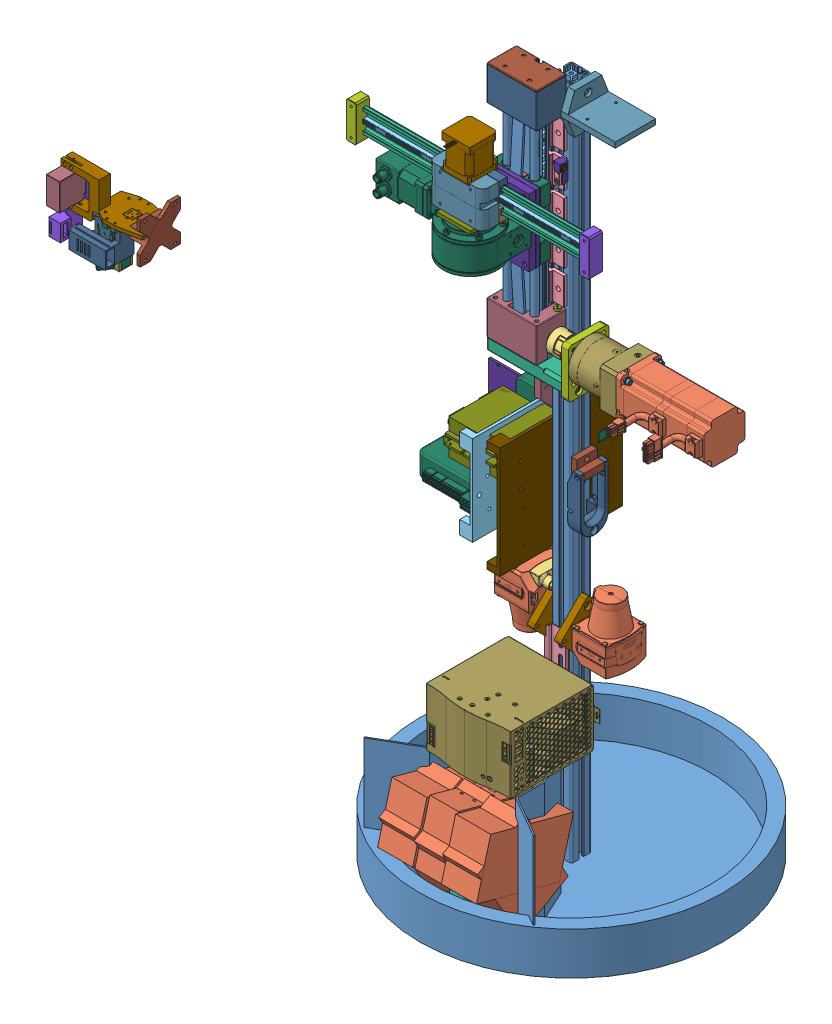
SolidWorks assembly Igus Axes Assembly, configuration Default. Lengths in mm.
Overall size (1488.85 1013 1350).
212 component instances, 89 part files, 64 mates.
Components (placement in the parent):
- Item Profile 6-1: Item Profile 6 [Default] at (483.1878 96.2857 998.7104) size (30 1000 30)
- TIM551 Lidar-1: TIM551 Lidar [Default] at (543.1878 396.2857 1000.2581) size (85.26 98.36 61.15)
  - TIM551 Lidar.igs-1: TIM551 Lidar.igs [Default] at origin size (85.26 98.36 61.15)
    - Assembly1.igs-1: Assembly1.igs [Default] at origin size (85.26 98.36 61.15)
      - 9194920_TiM55._56._35._36._Dummy.igs-1: 9194920_TiM55._56._35._36._Dummy.igs [Default] at origin size (85.26 98.36 61.15)
        - S105071_TiM55x_Mantelteile.igs-1: S105071_TiM55x_Mantelteile.igs [Default] at (11.3439 3.1936 0) x (0 1 0) z (0 0 -1) size (98.36 71.39 61.15)
        - S105072_TiM55x_Steckeranschluss_Dummy.igs-1: S105072_TiM55x_Steckeranschluss_Dummy.igs [Default] at (52.6134 34.7282 -20.9281) x (-1 0 0.000098) z (0.000098 -0.000098 1) size (37.21 29.83 42.7)
- Z Axis-1: Z Axis [Default] at (453.5786 1106.2857 1013.5104) x (1 0 0) z (0 -1 0) size (331.51 109.68 369.54)
  - D00684285.STEP-1: D00684285.STEP [Default] at origin size (331.51 109.68 369.54)
    - D00424608.iam.STEP-1: D00424608.iam.STEP [Default] at (0 0 52) x (-1 0 0) z (0 0 -1) size (74 44 56)
      - D00418189.iam.STEP-1: D00418189.iam.STEP [Default] at (0 22 30) x (-1 0 0) z (0 0 1) size (71 40 33.5)
        - D00160580.ipt.STEP-1: D00160580.ipt.STEP [Default] x (0 0 -1) z (-1 0 0) size (23 23 67.7)
        - D00129954.ipt.STEP-1: D00129954.ipt.STEP [Default] at (-25.5 0 0) x (0 1 0) z (-1 0 0) size (40 30 10)
        - D00129954.ipt.STEP-2: D00129954.ipt.STEP [Default] at (25.5 0 0) x (0 -1 0) z (1 0 0) size (40 30 10)
        - D00130409.ipt.STEP-1: D00130409.ipt.STEP [Default] at (-33.5 0 0) x (0 0 1) z (1 0 0) size (26 26 8)
        - D00130409.ipt.STEP-2: D00130409.ipt.STEP [Default] at (33.5 0 0) x (0 0 -1) z (-1 0 0) size (26 26 8)
        - D00130495.ipt.STEP-1: D00130495.ipt.STEP [Default] at (30.5 -15.5 -15) x (0 0 1) z (-1 0 0) size (23.5 8.5 8.5)
        - D00130495.ipt.STEP-2: D00130495.ipt.STEP [Default] at (-30.5 -15.5 -15) x (0 0 1) z (-1 0 0) size (23.5 8.5 8.5)
        - D00130495.ipt.STEP-3: D00130495.ipt.STEP [Default] at (-30.5 15.5 -15) x (0 0 1) z (-1 0 0) size (23.5 8.5 8.5)
        - D00130495.ipt.STEP-4: D00130495.ipt.STEP [Default] at (30.5 15.5 -15) x (0 0 1) z (1 0 0) size (23.5 8.5 8.5)
        - D00111820.ipt.STEP-1: D00111820.ipt.STEP [Default] at (-30.5 15.5 6.5896) x (0 0 1) z (1 0 0) size (5 5 5)
        - D00111820.ipt.STEP-2: D00111820.ipt.STEP [Default] at (-30.5 -15.5 6.5896) x (0 0 1) z (-1 0 0) size (5 5 5)
        - D00111820.ipt.STEP-3: D00111820.ipt.STEP [Default] at (30.5 -15.5 6.5896) x (0 0 1) z (-1 0 0) size (5 5 5)
        - D00111820.ipt.STEP-4: D00111820.ipt.STEP [Default] at (30.5 15.5 6.5896) x (0 0 1) z (-1 0 0) size (5 5 5)
      - D00129171.ipt.STEP-1: D00129171.ipt.STEP [Default] at (15 23.25 12) x (0 0 -1) z (1 0 0) size (18.8 7 7)
      - D00129171.ipt.STEP-2: D00129171.ipt.STEP [Default] at (-15 23.25 12) x (0 0 -1) z (1 0 0) size (18.8 7 7)
      - D00131296.ipt.STEP-1: D00131296.ipt.STEP [Default] x (-1 0 0) z (0 0 -1) size (74 44 50)
      - SAXT-104002.STEP-1: SAXT-104002.STEP [Default] at (0 22 52) x (-1 0 0) z (0 0 -1) size (74 44 7)
    - D00419202.iam.STEP-1: D00419202.iam.STEP [Default] at (0 0 302) size (94 44 56)
      - D00417520.iam.STEP-1: D00417520.iam.STEP [Default] at (0 22 25) x (-1 0 0) z (0 0 1) size (92.5 40 30)
        - D00130409.ipt.STEP-1: D00130409.ipt.STEP [Default] at (-25.5 0 0) x (0 -0.119291 0.992859) z (-1 0 0) size (26 26 8)
        - D00130409.ipt.STEP-2: D00130409.ipt.STEP [Default] at (33.5 0 0) x (0 0 -1) z (-1 0 0) size (26 26 8)
        - D00129954.ipt.STEP-1: D00129954.ipt.STEP [Default] at (-25.5 0 0) x (0 1 0) z (-1 0 0) size (40 30 10)
        - D00129954.ipt.STEP-2: D00129954.ipt.STEP [Default] at (25.5 0 0) x (0 -1 0) z (1 0 0) size (40 30 10)
        - D00160618.ipt.STEP-1: D00160618.ipt.STEP [Default] x (0 0 1) z (-1 0 0) size (23 23 90.85)
      - D00129171.ipt.STEP-1: D00129171.ipt.STEP [Default] at (15 23.25 12) x (0 0 -1) z (1 0 0) size (18.8 7 7)
      - D00129171.ipt.STEP-2: D00129171.ipt.STEP [Default] at (-15 23.25 12) x (0 0 -1) z (1 0 0) size (18.8 7 7)
      - D00130495.ipt.STEP-1: D00130495.ipt.STEP [Default] at (-30.5 6.5 0) x (0 0 1) z (-1 0 0) size (23.5 8.5 8.5)
      - D00130495.ipt.STEP-2: D00130495.ipt.STEP [Default] at (30.5 6.5 0) x (0 0 1) z (-1 0 0) size (23.5 8.5 8.5)
      - D00131302.ipt.STEP-1: D00131302.ipt.STEP [Default] x (-1 0 0) z (0 0 -1) size (74 44 50)
      - SAXT-104002_1.STEP-1: SAXT-104002_1.STEP [Default] at (0 22 52) x (-1 0 0) z (0 0 -1) size (74 44 24.04)
    - D00132325.iam.STEP-1: D00132325.iam.STEP [Default] at (0 30 177) size (73 22.56 100)
      - D00065372.iam.STEP-1: D00065372.iam.STEP [Default] at (-20 0 -35.5) size (26 17.3 29)
        - D00065332.ipt.STEP-1: D00065332.ipt.STEP [Default] at origin size (26 16.5 29)
        - D00346501.ipt.STEP-1: D00346501.ipt.STEP [Default] x (0.866025 0.5 0) z (0 0 1) size (13.08 12.43 28)
      - D00065372.iam.STEP-2: D00065372.iam.STEP [Default] at (-20 0 35.5) size (26 17.3 29)
        - D00065332.ipt.STEP-1: D00065332.ipt.STEP [Default] at origin size (26 16.5 29)
        - D00346501.ipt.STEP-1: D00346501.ipt.STEP [Default] x (0.866025 0.5 0) z (0 0 1) size (13.08 12.43 28)
      - D00065372.iam.STEP-3: D00065372.iam.STEP [Default] at (20 0 -35.5) x (-1 0 0) z (0 0 -1) size (26 17.3 29)
        - D00065332.ipt.STEP-1: D00065332.ipt.STEP [Default] at origin size (26 16.5 29)
        - D00346501.ipt.STEP-1: D00346501.ipt.STEP [Default] x (0.866025 0.5 0) z (0 0 1) size (13.08 12.43 28)
      - D00065372.iam.STEP-4: D00065372.iam.STEP [Default] at (20 0 35.5) x (-1 0 0) z (0 0 -1) size (26 17.3 29)
        - D00065332.ipt.STEP-1: D00065332.ipt.STEP [Default] at origin size (26 16.5 29)
        - D00346501.ipt.STEP-1: D00346501.ipt.STEP [Default] x (0.866025 0.5 0) z (0 0 1) size (13.08 12.43 28)
      - D00132323.ipt.STEP-1: D00132323.ipt.STEP [Default] at (0 9 0) size (73 6.52 100)
      - D00094049.ipt.STEP-1: D00094049.ipt.STEP [Default] at (30 10.5 27.5) x (0 -1 0) z (-0.000617 0 1) size (20 10 10)
      - D00094049.ipt.STEP-2: D00094049.ipt.STEP [Default] at (30 10.5 -27.5) x (0 -1 0) z (-0.000617 0 1) size (20 10 10)
      - D00094049.ipt.STEP-3: D00094049.ipt.STEP [Default] at (-30 10.5 27.5) x (0 -1 0) z (-0.000617 0 1) size (20 10 10)
      - D00094049.ipt.STEP-4: D00094049.ipt.STEP [Default] at (-30 10.5 -27.5) x (0 -1 0) z (-0.000617 0 1) size (20 10 10)
      - eBom-prt15.STEP-1: eBom-prt15.STEP [Default] at origin
    - D00506371.STEP-1: D00506371.STEP [Default] at (0 22 177) size (20.04 32.95 325.65)
      - D00506373.STEP-1: D00506373.STEP [Default] at origin size (16 26.8 325.65)
      - D00234495.ipt.STEP-1: D00234495.ipt.STEP [Default] at (0 9.875 -30) x (0 0 -1) z (1 0 0) size (40.02 8.02 20.02)
      - D00234495.ipt.STEP-2: D00234495.ipt.STEP [Default] at (0 9.875 30) x (0 0 1) z (-1 0 0) size (40.02 8.02 20.02)
      - D00133498.ipt.STEP-1: D00133498.ipt.STEP [Default] at (0 22.625 -17.5) x (0 -1 0) z (-0.999973 0 -0.007405) size (16 11.34 11.34)
      - D00133498.ipt.STEP-2: D00133498.ipt.STEP [Default] at (0 22.625 17.5) x (0 -1 0) z (-0.997414 0 0.071866) size (16 11.34 11.34)
    - D00308503.iam.STEP-1: D00308503.iam.STEP [Default] at (0 0 57) x (0 1 0) z (0 0 1) size (19.75 76.42 240)
      - D00308504.ipt.STEP-1: D00308504.ipt.STEP [Default] at (0.2 -12.5145 40) x (0 1 0) z (0 0 -1) size (27.65 8.9 40)
      - D00308504.ipt.STEP-2: D00308504.ipt.STEP [Default] at (0.2 12.5145 0) x (0 -1 0) z (0 0 1) size (27.65 8.9 40)
      - D00308504.ipt.STEP-3: D00308504.ipt.STEP [Default] at (0.2 -12.5145 90) x (0 1 0) z (0 0 -1) size (27.65 8.9 40)
      - D00308504.ipt.STEP-4: D00308504.ipt.STEP [Default] at (0.2 12.5145 50) x (0 -1 0) z (0 0 1) size (27.65 8.9 40)
      - D00308504.ipt.STEP-5: D00308504.ipt.STEP [Default] at (0.2 -12.5145 140) x (0 1 0) z (0 0 -1) size (27.65 8.9 40)
      - D00308504.ipt.STEP-6: D00308504.ipt.STEP [Default] at (0.2 12.5145 100) x (0 -1 0) z (0 0 1) size (27.65 8.9 40)
      - D00308504.ipt.STEP-7: D00308504.ipt.STEP [Default] at (0.2 -12.5145 190) x (0 1 0) z (0 0 -1) size (27.65 8.9 40)
      - D00308504.ipt.STEP-8: D00308504.ipt.STEP [Default] at (0.2 12.5145 150) x (0 -1 0) z (0 0 1) size (27.65 8.9 40)
      - D00308504.ipt.STEP-9: D00308504.ipt.STEP [Default] at (0.2 -12.5145 240) x (0 1 0) z (0 0 -1) size (27.65 8.9 40)
      - D00308504.ipt.STEP-10: D00308504.ipt.STEP [Default] at (0.2 12.5145 200) x (0 -1 0) z (0 0 1) size (27.65 8.9 40)
      - D00119001.ipt.STEP-1: D00119001.ipt.STEP [Default] at (15.25 -18.4 9.4087) x (0 0 -1) z (0 1 0) size (19.01 9 4)
      - D00119001.ipt.STEP-2: D00119001.ipt.STEP [Default] at (15.25 14.4 9.4087) x (0 0 -1) z (0 1 0) size (19.01 9 4)
      - D00119001.ipt.STEP-3: D00119001.ipt.STEP [Default] at (15.25 -18.4 29.4087) x (0 0 -1) z (0 1 0) size (19.01 9 4)
      - D00119001.ipt.STEP-4: D00119001.ipt.STEP [Default] at (15.25 14.4 29.4087) x (0 0 -1) z (0 1 0) size (19.01 9 4)
      - D00119001.ipt.STEP-5: D00119001.ipt.STEP [Default] at (15.25 -18.4 49.4087) x (0 0 -1) z (0 1 0) size (19.01 9 4)
      - D00119001.ipt.STEP-6: D00119001.ipt.STEP [Default] at (15.25 14.4 49.4087) x (0 0 -1) z (0 1 0) size (19.01 9 4)
      - D00119001.ipt.STEP-7: D00119001.ipt.STEP [Default] at (15.25 -18.4 69.4087) x (0 0 -1) z (0 1 0) size (19.01 9 4)
      - D00119001.ipt.STEP-8: D00119001.ipt.STEP [Default] at (15.25 14.4 69.4087) x (0 0 -1) z (0 1 0) size (19.01 9 4)
      - D00111820.ipt.STEP-1: D00111820.ipt.STEP [Default] at (15.25 13.4 9.4087) x (0 1 0) z (-0.18197 0 -0.983304) size (5 5 5)
      - D00111820.ipt.STEP-2: D00111820.ipt.STEP [Default] at (15.25 -13.4 9.4087) x (0 -1 0) z (0.628801 0 0.777566) size (5 5 5)
      - D00111820.ipt.STEP-3: D00111820.ipt.STEP [Default] at (15.25 13.4 29.4087) x (0 1 0) z (-0.18197 0 -0.983304) size (5 5 5)
      - D00111820.ipt.STEP-4: D00111820.ipt.STEP [Default] at (15.25 -13.4 29.4087) x (0 -1 0) z (0.628801 0 0.777566) size (5 5 5)
    - D00423744.iam.STEP-1: D00423744.iam.STEP [Default] at (30 22 342) size (138 60 72.54)
      - D00206252.ipt.STEP-1: D00206252.ipt.STEP [Default] at origin size (119 44 27.54)
      - D00210016.ipt.STEP-1: D00210016.ipt.STEP [Default] at (52 0 -15) x (0 -1 0) z (1 0 0) size (60 72.5 10)
      - D00094049.ipt.STEP-1: D00094049.ipt.STEP [Default] at (55 14 19) x (-1 0 0) z (0 0 -1) size (20 10 10)
      - D00095471.ipt.STEP-1: D00095471.ipt.STEP [Default] at (49.6 14 19) x (0 -1 0) z (0 0 -1) size (8 9.2 8)
      - D00094049.ipt.STEP-2: D00094049.ipt.STEP [Default] at (55 -14 19) x (-1 0 0) z (0 0 -1) size (20 10 10)
      - D00095471.ipt.STEP-2: D00095471.ipt.STEP [Default] at (49.6 -14 19) x (0 -1 0) z (0 0 -1) size (8 9.2 8)
      - D00206265.ipt.STEP-1: D00206265.ipt.STEP [Default] at (-60.5 15.5 18) x (0 0 -1) z (1 0 0) size (34.25 10 10)
      - D00206265.ipt.STEP-2: D00206265.ipt.STEP [Default] at (-60.5 -15.5 18) x (0 0 -1) z (1 0 0) size (34.25 10 10)
      - D00206265.ipt.STEP-3: D00206265.ipt.STEP [Default] at (0.5 15.5 18) x (0 0 -1) z (1 0 0) size (34.25 10 10)
      - D00206265.ipt.STEP-4: D00206265.ipt.STEP [Default] at (0.5 -15.5 18) x (0 0 -1) z (1 0 0) size (34.25 10 10)
      - D00095475.ipt.STEP-1: D00095475.ipt.STEP [Default] at (51 17.6777 -32.6777) size (1 10 10)
      - D00130495.ipt.STEP-1: D00130495.ipt.STEP [Default] at (51 17.6777 -32.6777) size (23.5 8.5 8.5)
      - D00025763.ipt.STEP-1: D00025763.ipt.STEP [Default] at (51 17.6777 -32.6777) size (21 8.5 8.5)
      - D00095475.ipt.STEP-2: D00095475.ipt.STEP [Default] at (51 17.6777 2.6777) x (1 0 0) z (0 -1 0) size (1 10 10)
      - D00130495.ipt.STEP-2: D00130495.ipt.STEP [Default] at (51 17.6777 2.6777) x (1 0 0) z (0 -1 0) size (23.5 8.5 8.5)
      - D00025763.ipt.STEP-2: D00025763.ipt.STEP [Default] at (51 17.6777 2.6777) x (1 0 0) z (0 -1 0) size (21 8.5 8.5)
      - D00095475.ipt.STEP-3: D00095475.ipt.STEP [Default] at (51 -17.6777 2.6777) x (1 0 0) z (0 0 -1) size (1 10 10)
      - D00130495.ipt.STEP-3: D00130495.ipt.STEP [Default] at (51 -17.6777 2.6777) x (1 0 0) z (0 0 -1) size (23.5 8.5 8.5)
      - D00025763.ipt.STEP-3: D00025763.ipt.STEP [Default] at (51 -17.6777 2.6777) x (1 0 0) z (0 0 -1) size (21 8.5 8.5)
      - D00095475.ipt.STEP-4: D00095475.ipt.STEP [Default] at (51 -17.6777 -32.6777) x (1 0 0) z (0 1 0) size (1 10 10)
      - D00130495.ipt.STEP-4: D00130495.ipt.STEP [Default] at (51 -17.6777 -32.6777) x (1 0 0) z (0 1 0) size (23.5 8.5 8.5)
      - D00025763.ipt.STEP-4: D00025763.ipt.STEP [Default] at (51 -17.6777 -32.6777) x (1 0 0) z (0 1 0) size (21 8.5 8.5)
    - D00439874.iam.STEP-1: D00439874.iam.STEP [Default] at (92 22 327) x (0 0 1) z (-1 0 0) size (60.02 60.04 120.8)
      - D00376785.ipt.STEP-1: D00376785.ipt.STEP [Default] at origin size (60.02 60.04 106)
      - D00474705.ipt.STEP-1: D00474705.ipt.STEP [Default] at (0 0 -48) x (0 1 0) z (0 0 -1) size (13.95 14 20.03)
      - D00109352.ipt.STEP-1: D00109352.ipt.STEP [Default] at (-23.582 23.582 -81.8) x (0 0 1) z (-1 0 0) size (16 7 7)
      - D00109352.ipt.STEP-2: D00109352.ipt.STEP [Default] at (23.582 23.582 -81.8) x (0 0 1) z (-1 0 0) size (16 7 7)
      - D00109352.ipt.STEP-3: D00109352.ipt.STEP [Default] at (-23.582 -23.582 -81.8) x (0 0 1) z (-1 0 0) size (16 7 7)
      - D00109352.ipt.STEP-4: D00109352.ipt.STEP [Default] at (23.582 -23.582 -81.8) x (0 0 1) z (-1 0 0) size (16 7 7)
      - D00100520.ipt.STEP-1: D00100520.ipt.STEP [Default] at (-23.582 23.582 -81.8) x (0 0 1) z (1 0 0) size (0.8 9 9)
      - D00100520.ipt.STEP-2: D00100520.ipt.STEP [Default] at (23.582 23.582 -81.8) x (0 0 1) z (1 0 0) size (0.8 9 9)
      - D00100520.ipt.STEP-3: D00100520.ipt.STEP [Default] at (-23.582 -23.582 -81.8) x (0 0 1) z (1 0 0) size (0.8 9 9)
      - D00100520.ipt.STEP-4: D00100520.ipt.STEP [Default] at (23.582 -23.582 -81.8) x (0 0 1) z (1 0 0) size (0.8 9 9)
    - D00265100.iam.STEP-1: D00265100.iam.STEP [Default] at (45.4 15.25 127.4087) x (-1 0 0) z (0 0 -1) size (15.5 12.2 27)
      - D00177454.ipt.STEP-1: D00177454.ipt.STEP [Default] at (1.5 5 4) x (0 -1 0) z (0.788943 0 -0.614466) size (10 5.6 5.54)
      - D00177453.ipt.STEP-1: D00177453.ipt.STEP [Default] at origin size (11 12.2 27)
      - D00129169.ipt.STEP-1: D00129169.ipt.STEP [Default] at (-1 0 21) size (15.5 8.5 8.5)
    - D00316386.STEP-1: D00316386.STEP [Default] at (0 0 42) size (50 35 270)
    - D00480302.ipt.STEP-1: D00480302.ipt.STEP [Default] at (163 22 327) x (0 0 1) z (-1 0 0) size (60.5 109.68 151.3)
    - D00416362.ipt.STEP-1: D00416362.ipt.STEP [Default] at (61 22 327) x (0 0 -1) z (1 0 0) size (32.02 32.01 32)
    - D00177460.ipt.STEP-1: D00177460.ipt.STEP [Default] at (43.9 16.75 111.4087) x (-1 0 0) z (0 1 0) size (8 23 4.7)
- X Axis-1: X Axis [Default] at (633.8286 994.2857 1102.7604) x (0 1 0) z (0 0 1) size (100 360.5 57.25)
  - GRW_0630_B_80_250_17_L_S_000_1.stp-1: GRW_0630_B_80_250_17_L_S_000_1.stp [Default] at origin size (100 360.5 57.25)
    - 2024_06_14_20_41_47_0760.stp-1: 2024_06_14_20_41_47_0760.stp [Default] at origin size (6 346.5 6.7)
    - 2024_06_14_20_41_47_0744.stp-1: 2024_06_14_20_41_47_0744.stp [Default] at origin size (35 346.5 10)
    - 2024_06_14_20_41_47_0729.stp-1: 2024_06_14_20_41_47_0729.stp [Default] at origin size (54 15 20)
    - 2024_06_14_20_41_47_0713.stp-1: 2024_06_14_20_41_47_0713.stp [Default] at origin size (54 15 20)
    - 2024_06_14_20_41_47_0697.stp-1: 2024_06_14_20_41_47_0697.stp [Default] at origin size (73 42 57)
    - 2024_06_14_20_41_47_0682.stp-1: 2024_06_14_20_41_47_0682.stp [Default] at origin size (18 19 12.5)
    - 2024_06_14_20_41_47_0666.stp-1: 2024_06_14_20_41_47_0666.stp [Default] at origin size (18 19 12.5)
    - 2024_06_14_20_41_47_0651.stp-1: 2024_06_14_20_41_47_0651.stp [Default] at origin size (18 19 12.5)
    - 2024_06_14_20_41_47_0635.stp-1: 2024_06_14_20_41_47_0635.stp [Default] at origin size (18 19 12.5)
    - 2024_06_14_20_41_47_0619.stp-1: 2024_06_14_20_41_47_0619.stp [Default] at origin size (54 80.5 42.5)
- Rotary Axis-1: Rotary Axis [Default] at (453.5786 930.7857 1068.5104) x (-1 0 0) z (0 0 1) size (190.51 53.01 92.26)
- Packaging sketch-1: Packaging sketch [Default] at (483.1878 96.2857 998.7104) size (1488.85 0 1350)
- rotary_x_connector-1: rotary_x_connector [Default] at (453.5786 963.7857 1118.7604) x (1 0 0) z (0 0 -1) size (50 70 50)
- rotary_z_connector_plate-1: rotary_z_connector_plate [Default] at (417.0786 979.2857 1058.5104) size (73 100 10)
- item_41967_angle-bracket-set-6-30x3__high-1: item_41967_angle-bracket-set-6-30x3__high [Default] at (423.9694 844.2857 1013.7104) size (30 39.71 39.71)
  - item_41967_angle-bracket-set-6-30x3__high.step-1: item_41967_angle-bracket-set-6-30x3__high.step [Default] at origin size (30 40.99 40.99) (hidden)
    - 2024_06_19_15_57_45_0002.step-1: 2024_06_19_15_57_45_0002.step [Default] at origin size (10.6 17 7.71)
    - 2024_06_19_15_57_44_0986.step-1: 2024_06_19_15_57_44_0986.step [Default] at origin size (10.6 7.71 17)
    - 2024_06_19_15_57_44_0970.step-1: 2024_06_19_15_57_44_0970.step [Default] at origin size (10.5 10.5 17.3)
    - 2024_06_19_15_57_44_0954.step-1: 2024_06_19_15_57_44_0954.step [Default] at origin size (10.5 17.3 10.5)
    - 2024_06_19_15_57_44_0939.step-1: 2024_06_19_15_57_44_0939.step [Default] at origin size (10.5 10.5 1.3)
    - 2024_06_19_15_57_44_0923.step-1: 2024_06_19_15_57_44_0923.step [Default] at origin size (10.5 1.3 10.5)
    - 2024_06_19_15_57_44_0907.step-1: 2024_06_19_15_57_44_0907.step [Default] at origin size (30 30.28 30.28) (hidden)
    - 2024_06_19_15_57_44_0891.step-1: 2024_06_19_15_57_44_0891.step [Default] at origin size (30 32.01 32.01)
- Item Profile 6- spacer-1: Item Profile 6- spacer [Default] at (468.1878 1029.3857 998.7104) x (0 1 0) z (0 0 1) size (30 50 30)
- Item Profile 6- spacer-2: Item Profile 6- spacer [Default] at (468.1878 829.2857 998.7104) x (0 1 0) z (0 0 1) size (30 50 30)
- Laser Mount-1: Laser Mount [Default] at (498.1878 396.2857 998.7104) x (0 0 -1) z (1 0 0) size (79.86 79.86 10)
- Laser Mount-2: Laser Mount [Default] at (458.1878 396.2857 998.7104) x (0 0 -1) z (1 0 0) size (79.86 79.86 10)
- TIM551 Lidar-2: TIM551 Lidar [Default] at (423.1878 422.4161 1000.2581) x (-1 0 0) z (0 0 1) size (85.26 98.36 61.15)
  - TIM551 Lidar.igs-1: TIM551 Lidar.igs [Default] at origin size (85.26 98.36 61.15)
    - Assembly1.igs-1: Assembly1.igs [Default] at origin size (85.26 98.36 61.15)
      - 9194920_TiM55._56._35._36._Dummy.igs-1: 9194920_TiM55._56._35._36._Dummy.igs [Default] at origin size (85.26 98.36 61.15)
        - S105071_TiM55x_Mantelteile.igs-1: S105071_TiM55x_Mantelteile.igs [Default] at (11.3439 3.1936 0) x (0 1 0) z (0 0 -1) size (98.36 71.39 61.15)
        - S105072_TiM55x_Steckeranschluss_Dummy.igs-1: S105072_TiM55x_Steckeranschluss_Dummy.igs [Default] at (52.6134 34.7282 -20.9281) x (-1 0 0.000098) z (0.000098 -0.000098 1) size (37.21 29.83 42.7)
- tagcameramounting1-1: tagcameramounting1 [Default] at (512.1878 588.6594 984.5604) x (0 -1 0) z (-1 0 0) size (86.47 41.25 19.85)
- tagcameramounting2^Igus Axes Assembly-1: tagcameramounting2^Igus Axes Assembly [Default] at (512.1878 588.6594 1013.8342) x (0 1 0) z (0 0 -1) size (22 19 30.25) (virtual)
- NDR-480-24-1: NDR-480-24 [Default] at (469.4866 257.5495 1126.5834) x (0 0 -1) z (1 0 0) size (139.51 85.5 128.91)
- netgear_mount_v1.stp-1: netgear_mount_v1.stp [Default] at (468.1878 726.2857 968.7104) x (0 0 1) z (-1 0 0) size (60 60 10.01)
- antenna_mount_v1.stp-1: antenna_mount_v1.stp [Default] at (498.1878 1096.2857 1028.7104) x (0 0 -1) z (1 0 0) size (60 60 80)
- Controller Box-1: Controller Box [Default] at (372.1557 675.8129 851.2554) x (1 0 0) z (0 -1 0) size (122.86 182.31 165)
  - D1_1-1: D1_1 [Default] at (87.0321 86.8 105.4604) size (122.86 31 139.6)
    - D1_1.stp-1: D1_1.stp [Default] at origin size (122.86 31 139.6)
      - 2024_06_27_15_43_33_0455.stp-1: 2024_06_27_15_43_33_0455.stp [Default] at origin size (122.86 31 139.6)
  - D7_2-1: D7_2 [Default] at (92.0321 163.45 68.5761) x (-1 0 0) z (0 0 -1) size (68.43 92.3 21)
    - D7_2.stp-1: D7_2.stp [Default] at origin size (68.43 92.3 21)
      - 2024_06_27_15_43_58_0075.stp-1: 2024_06_27_15_43_58_0075.stp [Default] at origin size (68.43 92.3 21)
  - D7_2-2: D7_2 [Default] at (92.0321 163.45 78.5761) x (-1 0 0) z (0 0 1) size (68.43 92.3 21)
    - D7_2.stp-1: D7_2.stp [Default] at origin size (68.43 92.3 21)
      - 2024_06_27_15_43_58_0075.stp-1: 2024_06_27_15_43_58_0075.stp [Default] at origin size (68.43 92.3 21)
  - Arduino Giga Mounting pts-1: Arduino Giga Mounting pts [Default] at (89.0321 169.08 141.2461) x (0 -1 0) z (0 0 -1) size (101.31 3 53.34)
  - Controller BOX Base^Controller Box-1: Controller BOX Base^Controller Box [Default] at (92.0321 86.8 105.4604) x (0 0 -1) z (1 0 0) size (165 182.31 19)
- Robotino Base Battery Plate-1: Robotino Base Battery Plate [Default] at (483.1878 96.2857 1058.7104) size (450 178 450)
- Battery Holder-1: Battery Holder [Default] at (483.1878 133.7857 1119.6181) x (0 -0.5 0.866025) z (0 0.866025 0.5) size (86 146.5 127.09)
- Battery Holder Mount-1: Battery Holder Mount [Default] at (483.1878 155.2857 1082.3791) x (0 0.866025 0.5) z (0 0.5 -0.866025) size (95.56 59.72 63.92)
- TS 35 7.5 DIN RAIL PERFORATED 1000mm CUT TO LENGTH-1: TS 35 7.5 DIN RAIL PERFORATED 1000mm CUT TO LENGTH [Default] at (483.1878 246.2857 1017.9804) x (0 0 1) z (0 -1 0) size (7.52 35 145)
- Controller Boxv2-1: Controller Boxv2 [Default] at (322.4161 445.9727 892.567) size (122.86 133 165)
  - D1_1-1: D1_1 [Default] at (87.0321 86.8 105.4604) size (122.86 31 139.6)
    - D1_1.stp-1: D1_1.stp [Default] at origin size (122.86 31 139.6)
      - 2024_06_27_15_43_33_0455.stp-1: 2024_06_27_15_43_33_0455.stp [Default] at origin size (122.86 31 139.6)
  - D7_2-1: D7_2 [Default] at (92.0321 143.3 121.8104) x (-1 0 0) z (0 -1 0) size (68.43 92.3 21)
    - D7_2.stp-1: D7_2.stp [Default] at origin size (68.43 92.3 21)
      - 2024_06_27_15_43_58_0075.stp-1: 2024_06_27_15_43_58_0075.stp [Default] at origin size (68.43 92.3 21)
  - D7_2-2: D7_2 [Default] at (92.0321 153.3 121.8104) x (-1 0 0) z (0 1 0) size (68.43 92.3 21)
    - D7_2.stp-1: D7_2.stp [Default] at origin size (68.43 92.3 21)
      - 2024_06_27_15_43_58_0075.stp-1: 2024_06_27_15_43_58_0075.stp [Default] at origin size (68.43 92.3 21)
  - Arduino Giga Mounting pts-1: Arduino Giga Mounting pts [Default] at (40.2521 148.97 58.6604) x (1 0 0) z (0 1 0) size (101.31 3 53.34)
  - Controller BOX Base^Controller Boxv2-1: Controller BOX Base^Controller Boxv2 [Default] at (92.0321 86.8 105.4604) x (0 0 -1) z (1 0 0) size (165 133 19)
- Battery Holder Mount 2-1: Battery Holder Mount 2 [Default] at origin size (108.73 65.41 130.32)
- Battery Holder-2: Battery Holder [Default] at (483.1878 183.495 1094.12) x (0 0.965926 -0.258819) z (0 0.258819 0.965926) size (86 146.5 127.09)
- Gripper Assembly-1: Gripper Assembly [Default] at (37.5314 844.2928 1221.8311) x (0 0 -1) z (1 0 0) size (73.1 113.8 126.33)
  - back_fin-1: back_fin [Default] at (-39.1945 0.036 28.6679) x (-1 0 0) z (0 0 -1) size (42.34 68.5 19.17) (hidden)
  - fin_triangular-1: fin_triangular [Default] at (-39.7621 -51.964 -10.9821) x (0 1 0) z (0 0 -1) size (76.98 62.22 23.12)
  - mount_a-1: mount_a [Default] at (-39.2621 3.036 28.6679) size (56 59.3 120.65)
  - mount_b-1: mount_b [Default] at (-39.2621 3.036 40.7115) size (70.5 45 54)
  - mount_d-1: mount_d [Default] at (-39.2621 3.036 63.6689) size (60 60 23.18)
  - mount_c-1: mount_c [Default] at (-39.2621 3.036 16.6243) size (56 69 7) (hidden)
  - servomotor_mg996r-1: servomotor_mg996r [Default] at (-82.3621 -1.964 -27.4821) x (0 1 0) z (0 0 -1) size (53.6 47.6 20)
  - back_fin v2-1: back_fin v2 [Default] at (-39.1945 0.036 28.6679) x (-1 0 0) z (0 0 -1) size (42.34 68.5 19.17)
  - mount_c v2-1: mount_c v2 [Default] at (-39.2621 3.036 16.6243) size (56 69 22.2)
Mates (geometry in assembly coordinates):
- Distance2: distance = 0 mm anti-aligned: plane of Z Axis-1/D00684285.STEP-1/D00308503.iam.STEP-1/D00308504.ipt.STEP-3 through (472.5878 959.2857 1013.7104) normal (0 0 -1); plane of Item Profile 6-1 through (486.7878 1096.2857 1013.7104) normal (0 0 1)
- Distance3: distance = 3.1 mm: cylinder of Z Axis-1/D00684285.STEP-1/D00308503.iam.STEP-1/D00308504.ipt.STEP-9 through (483.1878 829.2857 1017.3104) axis (0 0 1) radius 3.2; plane of Item Profile 6-1 through (480.0878 1096.2857 1011.2104) normal (1 0 0)
- Coincident4: coincident: plane of ? through (483.1878 96.2857 998.7104) normal (0 0 1); point of ?
- Coincident5: coincident: plane of Item Profile 6-1 through (483.1878 96.2857 998.7104) normal (0 1 0)
- Coincident6: coincident: plane of Item Profile 6-1 through (483.1878 96.2857 998.7104) normal (1 0 0)
- Concentric6: concentric anti-aligned: cylinder of X Axis-1/GRW_0630_B_80_250_17_L_S_000_1.stp-1/2024_06_14_20_41_47_0619.stp-1 through (463.5786 1015.5357 1103.2604) axis (0 0 -1) radius 1.66; cylinder of rotary_x_connector-1 through (463.5786 1015.5357 1087.3245) axis (0 0 1) radius 1.65
- Concentric7: concentric anti-aligned: cylinder of X Axis-1/GRW_0630_B_80_250_17_L_S_000_1.stp-1/2024_06_14_20_41_47_0619.stp-1 through (443.5786 973.0357 1103.2604) axis (0 0 -1) radius 1.66; cylinder of rotary_x_connector-1 through (443.5786 973.0357 1087.3245) axis (0 0 1) radius 1.65
- Coincident8: coincident anti-aligned: plane of X Axis-1/GRW_0630_B_80_250_17_L_S_000_1.stp-1/2024_06_14_20_41_47_0619.stp-1 through (453.5786 1021.2857 1098.7604) normal (0 0 -1); plane of rotary_x_connector-1 through (468.5786 958.7857 1098.7604) normal (0 0 1)
- Concentric11: concentric anti-aligned: cylinder of Rotary Axis-1 through (453.5786 952.7857 1134.2604) axis (0 -1 0) radius 2.5; cylinder of rotary_x_connector-1 through (453.5786 958.0107 1134.2604) axis (0 1 0) radius 2.5
- Concentric12: concentric anti-aligned: cylinder of Rotary Axis-1 through (467.002 952.7857 1111.0104) axis (0 -1 0) radius 2.5; cylinder of rotary_x_connector-1 through (467.002 958.0107 1111.0104) axis (0 1 0) radius 2.5
- Concentric13: concentric anti-aligned: cylinder of Rotary Axis-1 through (440.1552 952.7857 1111.0104) axis (0 -1 0) radius 2.5; cylinder of rotary_x_connector-1 through (440.1552 958.0107 1111.0104) axis (0 1 0) radius 2.5
- Coincident9: coincident anti-aligned: plane of Rotary Axis-1 through (453.5786 958.7857 1098.7104) normal (0 1 0); plane of rotary_x_connector-1 through (453.5786 958.7857 1118.7604) normal (0 -1 0)
- Concentric15: concentric aligned: cylinder of Z Axis-1/D00684285.STEP-1/D00132325.iam.STEP-1/D00132323.ipt.STEP-1 through (483.5786 885.7857 934.5296) axis (0 0 1) radius 3.3; cylinder of rotary_z_connector_plate-1 through (483.5786 885.7857 1056.9604) axis (0 0 1) radius 3.2
- Concentric16: concentric aligned: cylinder of Z Axis-1/D00684285.STEP-1/D00132325.iam.STEP-1/D00132323.ipt.STEP-1 through (423.5786 972.7857 934.5296) axis (0 0 1) radius 3.3; cylinder of rotary_z_connector_plate-1 through (423.5786 972.7857 1056.9604) axis (0 0 1) radius 3.2
- Distance4: distance = 0 mm anti-aligned: cylinder of Z Axis-1/D00684285.STEP-1/D00132325.iam.STEP-1/D00132323.ipt.STEP-1 through (423.5786 929.2857 758.5104) axis (0 -1 0) radius 300; plane of rotary_z_connector_plate-1 through (417.0786 979.2857 1058.5104) normal (0 0 -1)
- Concentric19: concentric aligned: cylinder of Z Axis-1/D00684285.STEP-1/D00308503.iam.STEP-1/D00308504.ipt.STEP-10 through (423.9694 829.2857 1017.3104) axis (0 0 1) radius 3.2; cylinder of item_41967_angle-bracket-set-6-30x3__high-1/item_41967_angle-bracket-set-6-30x3__high.step-1/2024_06_19_15_57_44_0970.step-1 through (423.9694 829.2857 1016.5354) axis (0 0 1) radius 3
- Coincident11: coincident anti-aligned: plane of Z Axis-1/D00684285.STEP-1/D00308503.iam.STEP-1/D00308504.ipt.STEP-10 through (434.5694 849.2857 1013.7104) normal (0 0 -1); plane of item_41967_angle-bracket-set-6-30x3__high-1/item_41967_angle-bracket-set-6-30x3__high.step-1/2024_06_19_15_57_44_0891.step-1 through (408.9694 829.5357 1013.7104) normal (0 0 1)
- Concentric21: concentric anti-aligned: cylinder of Rotary Axis-1 through (473.5786 938.7857 1074.5104) axis (0 0 1) radius 1.621; cylinder of rotary_z_connector_plate-1 through (473.5786 938.7857 1069.9464) axis (0 0 -1) radius 1.65
- Concentric22: concentric aligned: cylinder of Rotary Axis-1 through (433.5786 922.7857 1074.5104) axis (0 0 1) radius 1.621; cylinder of rotary_z_connector_plate-1 through (433.5786 922.7857 1058.5104) axis (0 0 1) radius 1.5
- Coincident12: coincident anti-aligned: plane of Rotary Axis-1 through (433.8536 948.2857 1068.5104) normal (0 0 -1); plane of rotary_z_connector_plate-1 through (417.0786 979.2857 1068.5104) normal (0 0 1)
- Distance5: distance = 45 mm aligned: plane of X Axis-1/GRW_0630_B_80_250_17_L_S_000_1.stp-1/2024_06_14_20_41_47_0760.stp-1 through (453.5786 991.2857 1110.1104) normal (0 -1 0); plane of Item Profile 6-1 through (483.1878 946.2857 998.7104) normal (0 -1 0)
- Distance6: distance = 0 mm anti-aligned: plane of Item Profile 6- spacer-1 through (468.1878 1041.8857 1004.8104) normal (1 0 0); plane of Item Profile 6-1 through (468.1878 1096.2857 986.7104) normal (-1 0 0)
- Coincident16: coincident aligned: plane of Item Profile 6-1 through (495.1878 1096.2857 983.7104) normal (0 0 -1); plane of Item Profile 6- spacer-1 through (418.1878 1041.3857 983.7104) normal (0 0 -1)
- Distance7: distance = 0 mm anti-aligned: cylinder of Z Axis-1/D00684285.STEP-1/D00308503.iam.STEP-1/D00308504.ipt.STEP-2 through (423.9694 1029.2857 1017.3104) axis (0 0 1) radius 3.2; plane of Item Profile 6- spacer-1 through (418.1878 1032.4857 1011.2104) normal (0 -1 0)
- Coincident17: coincident anti-aligned: plane of Item Profile 6-1 through (468.1878 1096.2857 986.7104) normal (-1 0 0); plane of Item Profile 6- spacer-2 through (468.1878 841.7857 1004.8104) normal (1 0 0)
- Coincident18: coincident aligned: plane of Item Profile 6-1 through (495.1878 1096.2857 983.7104) normal (0 0 -1); plane of Item Profile 6- spacer-2 through (418.1878 841.2857 983.7104) normal (0 0 -1)
- Distance8: distance = 3.1 mm: cylinder of Z Axis-1/D00684285.STEP-1/D00308503.iam.STEP-1/D00308504.ipt.STEP-10 through (423.9694 829.2857 1017.3104) axis (0 0 1) radius 3.2; plane of Item Profile 6- spacer-2 through (418.1878 826.1857 1011.2104) normal (0 1 0)
- Coincident19: coincident anti-aligned: plane of Item Profile 6-1 through (498.1878 1096.2857 1010.7104) normal (1 0 0); plane of Laser Mount-1 through (498.1878 396.2857 998.7104) normal (-1 0 0)
- Distance9: distance = 3.1 mm: cylinder of Laser Mount-1 through (508.1878 424.57 998.7104) axis (1 0 0) radius 3.3; plane of Item Profile 6-1 through (497.6878 1096.2857 995.6104) normal (0 0 1)
- Distance10: distance = 35 mm aligned: plane of TIM551 Lidar-1/TIM551 Lidar.igs-1 through (543.1878 396.2857 1000.2581) normal (1 0 0); plane of Laser Mount-1 through (508.1878 396.2857 998.7104) normal (1 0 0)
- Coincident21: coincident aligned: plane of TIM551 Lidar-1 through (543.1878 396.2857 1000.2581) normal (0 1 0); plane of Laser Mount-1 through (498.1878 396.2857 998.7104) normal (0 1 0)
- Distance11: distance = 50 mm anti-aligned: plane of Laser Mount-1 through (498.1878 396.2857 998.7104) normal (0 1 0); plane of Item Profile 6-1 through (483.1878 346.2857 998.7104) normal (0 -1 0)
- Distance12: distance = 0 mm: cylinder of tagcameramounting1-1 through (517.6878 526.2857 998.7104) axis (1 0 0) radius 5.5; plane of Item Profile 6-1 through (483.1878 526.2857 998.7104) normal (0 -1 0)
- Coincident25: coincident anti-aligned: plane of Item Profile 6-1 through (498.1878 1096.2857 1010.7104) normal (1 0 0); plane of tagcameramounting1-1 through (498.1878 588.6594 984.5604) normal (-1 0 0)
- Distance13: distance = 3.1 mm: cylinder of tagcameramounting1-1 through (517.6878 526.2857 998.7104) axis (1 0 0) radius 3.3; plane of Item Profile 6-1 through (497.6878 1096.2857 1001.8104) normal (0 0 -1)
- InPlace1: in place: plane of tagcameramounting1-1 through (517.6878 606.6594 1013.8342) normal (0 0 -1); plane of ? through (0 0 1013.8342) normal (0 0 -1); moOrthogonalPlaneRef_w of tagcameramounting1-1 through (517.6878 606.6594 1013.8342) normal (0 0 -1); plane of ? through (0 0 1013.8342) normal (0 1 0); plane of tagcameramounting1-1 through (517.6878 606.6594 1013.8342) normal (0 0 -1); plane of ? through (0 0 1013.8342) normal (-1 0 0); plane of tagcameramounting1-1 through (517.6878 606.6594 1013.8342) normal (0 0 -1); unknown of tagcameramounting2^Igus Axes Assembly-1
- Coincident26: coincident aligned: plane of tagcameramounting1-1; plane of tagcameramounting2^Igus Axes Assembly-1
- Coincident27: coincident aligned: moOrthogonalPlaneRef_w of tagcameramounting1-1 through (512.1878 588.6594 1013.8342) normal (1 0 0); plane of tagcameramounting2^Igus Axes Assembly-1 through (512.1878 588.6594 1013.8342) normal (1 0 0)
- Coincident28: coincident anti-aligned: moOrthogonalPlaneRef_w of tagcameramounting1-1 through (512.1878 588.6594 1013.8342) normal (0 -1 0); plane of tagcameramounting2^Igus Axes Assembly-1 through (512.1878 588.6594 1013.8342) normal (0 1 0)
- Distance16: distance = 5.5 mm aligned: plane of NDR-480-24-1 through (469.4866 270.7857 1138.4504) normal (0 -1 0); plane of Item Profile 6-1 through (483.1878 276.2857 998.7104) normal (0 -1 0)
- Coincident27: coincident anti-aligned: plane of Item Profile 6-1 through (498.1878 1096.2857 986.7104) normal (1 0 0); plane of antenna_mount_v1.stp-1 through (498.1878 1096.2857 1028.7104) normal (-1 0 0)
- Distance18: distance = 3.1 mm: cylinder of antenna_mount_v1.stp-1 through (496.6378 1083.7857 998.7104) axis (1 0 0) radius 2.625; plane of Item Profile 6-1 through (497.6878 1096.2857 1001.8104) normal (0 0 -1)
- Distance19: distance = 0 mm aligned: plane of antenna_mount_v1.stp-1 through (498.1878 1096.2857 968.7104) normal (0 1 0); plane of Item Profile 6-1 through (495.6878 1096.2857 1004.8104) normal (0 1 0)
- Coincident29: coincident anti-aligned: plane of Item Profile 6-1 through (468.1878 1096.2857 1010.7104) normal (-1 0 0); plane of netgear_mount_v1.stp-1 through (468.1878 726.2857 968.7104) normal (1 0 0)
- Distance20: distance = 3.1 mm: cylinder of netgear_mount_v1.stp-1 through (469.7378 713.7857 998.7104) axis (-1 0 0) radius 2.625; plane of Item Profile 6-1 through (468.6878 1096.2857 995.6104) normal (0 0 1)
- Distance21: distance = 120 mm anti-aligned: plane of netgear_mount_v1.stp-1 through (468.1878 726.2857 1028.7104) normal (0 1 0); plane of Item Profile 6-1 through (483.1878 846.2857 998.7104) normal (0 -1 0)
- Coincident31: coincident anti-aligned: plane of Item Profile 6-1 through (468.1878 1096.2857 1010.7104) normal (-1 0 0); plane of Controller Box-1/Controller BOX Base^Controller Box-1 through (468.1878 570.3525 938.0554) normal (1 0 0)
- Distance22: distance = 3.1 mm: cylinder of Controller Box-1/Controller BOX Base^Controller Box-1 through (468.1888 642.8525 998.7104) axis (-1 0 0) radius 3.1; plane of Item Profile 6-1 through (468.6878 1096.2857 995.6104) normal (0 0 1)
- Distance24: distance = 60 mm anti-aligned: plane of Robotino Base Battery Plate-1 through (483.1878 271.2857 1058.7104) normal (0 0 -1); plane of Item Profile 6-1 through (483.1878 96.2857 998.7104) normal (0 0 1)
- Coincident34: coincident aligned: plane of Item Profile 6-1 through (483.1878 96.2857 998.7104) normal (1 0 0); plane of Robotino Base Battery Plate-1 through (483.1878 96.2857 1058.7104) normal (1 0 0)
- Coincident37: coincident aligned: plane of Item Profile 6-1 through (483.1878 96.2857 998.7104) normal (1 0 0); plane of Battery Holder-1 through (483.1878 133.7857 1119.6181) normal (1 0 0)
- Angle5: planar angle = 0.523599 rad anti-aligned: plane of Battery Holder-1 through (461.9378 248.8164 1136.3791) normal (0 0.5 -0.866025); plane of Robotino Base Battery Plate-1 through (483.1878 271.2857 1060.7104) normal (0 0 1)
- InPlace2: in place: plane of Battery Holder-1 through (461.9378 248.8164 1136.3791) normal (0 0.5 -0.866025); plane of ? through (0 -429.8625 744.5436) normal (0 0.5 -0.866025); plane of Battery Holder-1 through (461.9378 248.8164 1136.3791) normal (0 0.5 -0.866025); plane of ? through (0 -429.8625 744.5436) normal (0 0.866025 0.5); plane of Battery Holder-1 through (461.9378 248.8164 1136.3791) normal (0 0.5 -0.866025); plane of ? through (0 -429.8625 744.5436) normal (-1 0 0); plane of Battery Holder-1 through (461.9378 248.8164 1136.3791) normal (0 0.5 -0.866025); unknown of Battery Holder Mount-1
- Coincident39: coincident aligned: plane of Battery Holder-1; plane of Battery Holder Mount-1
- Coincident40: coincident aligned: moOrthogonalPlaneRef_w of Battery Holder-1 through (483.1878 155.2857 1082.3791) normal (1 0 0); plane of Battery Holder Mount-1 through (483.1878 155.2857 1082.3791) normal (1 0 0)
- Coincident41: coincident anti-aligned: moOrthogonalPlaneRef_w of Battery Holder-1 through (483.1878 155.2857 1082.3791) normal (0 -0.866025 -0.5); plane of Battery Holder Mount-1 through (483.1878 155.2857 1082.3791) normal (0 0.866025 0.5)
- Distance26: distance = 40 mm aligned: plane of TS 35 7.5 DIN RAIL PERFORATED 1000mm CUT TO LENGTH-1 through (469.6678 246.2857 1016.0004) normal (0 -1 0); plane of NDR-480-24-1 through (459.6866 286.2857 1078.176) normal (0 -1 0)
- Coincident43: coincident anti-aligned: plane of NDR-480-24-1 through (466.0268 345.6857 1021.2304) normal (0 0 -1); plane of TS 35 7.5 DIN RAIL PERFORATED 1000mm CUT TO LENGTH-1 through (470.6878 1246.2857 1021.2304) normal (0 0 1)
- Coincident44: coincident anti-aligned: plane of NDR-480-24-1 through (500.6878 345.6857 1020.7304) normal (-1 0 0); plane of TS 35 7.5 DIN RAIL PERFORATED 1000mm CUT TO LENGTH-1 through (500.6878 1246.2857 1021.2304) normal (1 0 0)
- Coincident45: coincident anti-aligned: plane of Item Profile 6-1 through (486.7878 1096.2857 1013.7104) normal (0 0 1); plane of TS 35 7.5 DIN RAIL PERFORATED 1000mm CUT TO LENGTH-1 through (495.6878 1246.2857 1013.7104) normal (0 0 -1)
- Distance28: distance = 3.1 mm: cylinder of TS 35 7.5 DIN RAIL PERFORATED 1000mm CUT TO LENGTH-1 through (483.1878 384.2857 1013.7104) axis (0 0 1) radius 3; plane of Item Profile 6-1 through (486.2878 1096.2857 1011.2104) normal (-1 0 0)
- Angle8: planar angle = 1.832596 rad aligned: plane of Battery Holder-2 through (504.4378 252.9823 1187.3108) normal (0 0.965926 -0.258819); plane of Robotino Base Battery Plate-1 through (483.1878 271.2857 1060.7104) normal (0 0 1)
- Coincident48: coincident anti-aligned: plane of Robotino Base Battery Plate-1 through (483.1878 96.2857 1058.7104) normal (1 0 0); plane of Battery Holder-2 through (483.1878 183.495 1094.12) normal (-1 0 0)
- Distance29: distance = 8 mm: plane of Robotino Base Battery Plate-1 through (483.1878 271.2857 1060.7104) normal (0 0 1); line of Battery Holder-2 through (409.9378 219.1329 1068.7104) axis (1 0 0)
